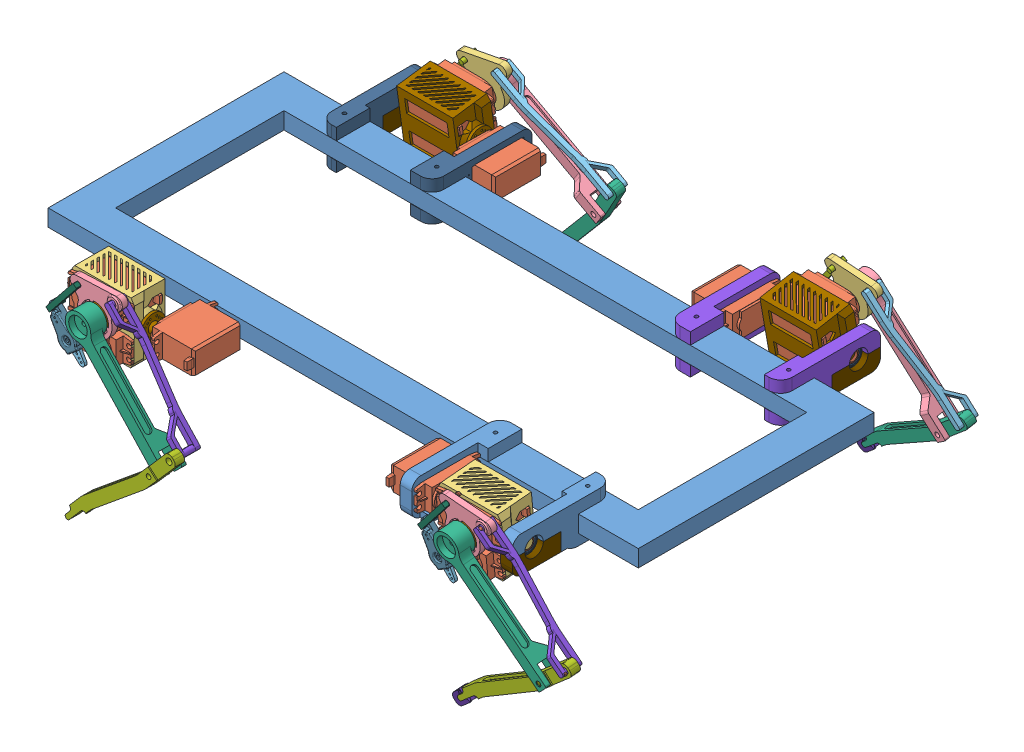
SolidWorks assembly Main Robot Assembly, configuration Default. Lengths in mm.
Overall size (614.33 209.08 462.35).
127 component instances, 28 part files, 12 mates.
Components (placement in the parent):
- Canvas Dimensions-1: Canvas Dimensions [Default] at (344.428 262.5412 316.9027) size (508 14.5 203)
- Robot Assembly-1: Robot Assembly [Default] at (-142.6556 246.9594 574.0725) x (-1 0 0) z (0 0.999972 -0.007524) size (279.4 91.93 183.61) (flexible)
  - MG996R-1: MG996R [Default] at (-78.3336 -28.8336 37.8009) size (54.5 42.75 20)
  - MG996R-2: MG996R [Default] at (-78.3336 -28.8336 11.8009) x (-1 0 0) z (0 0 -1) size (54.5 42.75 20)
  - MG996R-3: MG996R [Default] at (-152.8336 -26.2341 24.7786) x (0 -0.999972 0.007524) z (0 0.007524 0.999972) size (54.5 42.75 20)
  - Servo Housing-1: Servo Housing [Default] at (-78.3336 0.9164 37.8009) x (1 0 0) z (0 1 0) size (61.5 52 29.25)
  - Rotating Piece-1: Rotating Piece [Default] at (-88.8336 10.9164 37.9023) x (0.272127 0 -0.962261) z (0.962261 0 0.272127) size (44.28 6 43.21)
  - Double_Blade_Rudder-1: Double_Blade_Rudder [默认] at (-67.8336 16.2164 11.6996) x (0.777995 0 -0.62827) z (-0.62827 0 -0.777995) size (12.2 5.5 38)
  - Upper Leg-1: Upper Leg [Default] at (-164.7696 20.2164 -34.7892) x (-0.725082 0 0.688662) z (0 1 0) size (22 116.4 18)
  - Lower leg-1: Lower leg [Default] at (-80.9738 38.0729 -100.4378) x (0.753928 0 0.656957) z (0 -1 0) size (20.21 126 9.59)
  - Long Connection Rod-1: Long Connection Rod [Default] at (-101.7266 10.9164 56.8385) x (0.725085 0 -0.688659) z (-0.688659 0 -0.725085) size (5 22 105.4)
  - Circle Rudder-1: Circle Rudder [默认] at (-105.5836 -15.7336 24.8009) x (0 0.704253 -0.709949) z (0 0.709949 0.704253) size (20.8 5.5 20.8)
  - 688ZZ Bearing Assembly-2: 688ZZ Bearing Assembly [Default] at (-46.5836 -15.7336 24.8009) x (0 -0.986239 -0.165327) z (1 0 0) size (17.99 17.98 5)
    - Outer Ring-1: Outer Ring [Default] at origin size (16 16 5)
    - Inner Ring-1: Inner Ring [Default] x (-0.241565 -0.970385 0) z (0 0 1) size (10.6 10.6 5)
    - Cage-1: Cage [Default] x (0.535517 0.844524 0) z (0 0 1) size (13.01 13.06 2.21)
    - 2mm Ball Bearing-1: 2mm Ball Bearing [Default] at (-5.0671 3.2131 0) x (0.050652 0.835774 0.546732) z (0.977207 -0.154478 0.145614) size (2 2 2)
    - 2mm Ball Bearing-2: 2mm Ball Bearing [Default] at (-5.988 -0.3789 0) x (-0.450278 0.705928 0.546732) z (0.881377 0.449412 0.145614) size (2 2 2)
    - 2mm Ball Bearing-3: 2mm Ball Bearing [Default] at (-4.6217 -3.8262 0) x (-0.779216 0.306441 0.546732) z (0.448891 0.881642 0.145614) size (2 2 2)
    - 2mm Ball Bearing-4: 2mm Ball Bearing [Default] at (-1.49 -5.812 0) x (-0.810521 -0.210096 0.546732) z (-0.155056 0.977115 0.145614) size (2 2 2)
    - 2mm Ball Bearing-5: 2mm Ball Bearing [Default] at (2.2108 -5.5778 0) x (-0.532234 -0.646383 0.546732) z (-0.699777 0.699363 0.145614) size (2 2 2)
    - 2mm Ball Bearing-6: 2mm Ball Bearing [Default] at (5.0671 -3.2131 0) x (-0.050652 -0.835774 0.546732) z (-0.977207 0.154478 0.145614) size (2 2 2)
    - 2mm Ball Bearing-7: 2mm Ball Bearing [Default] at (5.988 0.3789 0) x (0.450278 -0.705928 0.546732) z (-0.881377 -0.449412 0.145614) size (2 2 2)
    - 2mm Ball Bearing-8: 2mm Ball Bearing [Default] at (4.6217 3.8262 0) x (0.779216 -0.306441 0.546732) z (-0.448891 -0.881642 0.145614) size (2 2 2)
    - 2mm Ball Bearing-9: 2mm Ball Bearing [Default] at (1.49 5.812 0) x (0.810521 0.210096 0.546732) z (0.155056 -0.977115 0.145614) size (2 2 2)
    - 2mm Ball Bearing-10: 2mm Ball Bearing [Default] at (-2.2108 5.5778 0) x (0.532234 0.646383 0.546732) z (0.699777 -0.699363 0.145614) size (2 2 2)
  - Circle Rudder-3: Circle Rudder [默认] at (-88.8336 16.2164 37.9023) x (-0.701297 0 -0.712869) z (-0.712869 0 0.701297) size (20.8 5.5 20.8)
  - Servo Arm Mount-1: Servo Arm Mount [Default] at (-67.8336 16.2164 11.6996) x (-0.777995 0 0.62827) z (0 1 0) size (16.2 34.39 7.06)
  - Short Connecting Rod-1: Short Connecting Rod [Default] at (-51.1485 16.2164 29.347) x (-0.625385 0 0.780316) z (0 1 0) size (37.08 4 13)
  - 91595A167_Dowel Pin-1: 91595A167_Dowel Pin [91595A167] at (-157.9784 20.8164 -34.8994) x (-0.98004 0 -0.198802) z (0 -1 0) size (4 4 20)
- Rear Robot Assembly-1: Rear Robot Assembly [Default] at (318.8891 198.8409 650.2972) x (-0.962615 -0.122983 0.241344) z (-0.105199 0.990787 0.085287) size (170.41 148.65 173.65) (flexible)
  - MG996R-1: MG996R [Default] at (29.5952 -122.5628 58.2658) x (-0.962615 0.249609 -0.105199) z (0.100626 -0.031047 -0.99444) size (54.5 42.75 20)
  - MG996R-2: MG996R [Default] at (26.9789 -121.7556 84.1213) x (0.962615 -0.249609 0.105199) z (-0.100626 0.031047 0.99444) size (54.5 42.75 20)
  - MG996R-3: MG996R [Default] at (100.7498 -138.2322 78.1733) x (-0.241344 -0.966685 -0.085287) z (0.122983 0.056709 -0.990787) size (54.5 42.75 20)
  - Servo Housing-1: Servo Housing [Default] at (37.077 -93.7693 58.1239) x (-0.962615 0.249609 -0.105199) z (0.251487 0.967849 -0.00477) size (61.5 52 29.25)
  - Rotating Piece-1: Rotating Piece [Default] at (26.8579 -80.6595 82.9278) x (0.47519 -0.127764 -0.870558) z (0.843178 -0.216668 0.492043) size (44.28 6 43.21)
  - Double_Blade_Rudder-1: Double_Blade_Rudder [默认] at (51.0424 -81.5852 59.0548) x (0.874959 -0.229452 -0.426377) z (-0.413763 0.103055 -0.904533) size (12.2 5.5 38)
  - Upper Leg-1: Upper Leg [Default] at (-40.9774 -53.7999 6.6799) x (-0.731758 0.193362 0.65356) z (0.251487 0.967849 -0.00477) size (22 116.4 18)
  - Lower leg-1: Lower leg [Default] at (54.3425 -73.1084 -38.5951) x (0.559538 -0.141367 0.816659) z (-0.251487 -0.967849 0.00477) size (20.21 126 9.59)
  - Long Connection Rod-1: Long Connection Rod [Default] at (10.5252 -76.3432 97.6098) x (0.731755 -0.193361 -0.653564) z (-0.633473 0.160873 -0.756856) size (5 22 105.4)
  - Circle Rudder-1: Circle Rudder [默认] at (57.8128 -116.2822 73.9977) x (0.107242 0.707834 0.698191) z (0.248738 0.660808 -0.70814) size (20.8 5.5 20.8)
  - 688ZZ Bearing Assembly-2: 688ZZ Bearing Assembly [Default] at (1.0185 -101.5553 67.791) x (-0.264501 -0.949925 0.166376) z (-0.962615 0.249609 -0.105199) size (17.99 17.98 5)
    - Outer Ring-1: Outer Ring [Default] at origin size (16 16 5)
    - Inner Ring-1: Inner Ring [Default] x (-0.241565 -0.970385 0) z (0 0 1) size (10.6 10.6 5)
    - Cage-1: Cage [Default] x (0.535517 0.844524 0) z (0 0 1) size (13.01 13.06 2.21)
    - 2mm Ball Bearing-1: 2mm Ball Bearing [Default] at (-5.0671 3.2131 0) x (0.050652 0.835774 0.546732) z (0.977207 -0.154478 0.145614) size (2 2 2)
    - 2mm Ball Bearing-2: 2mm Ball Bearing [Default] at (-5.988 -0.3789 0) x (-0.450278 0.705928 0.546732) z (0.881377 0.449412 0.145614) size (2 2 2)
    - 2mm Ball Bearing-3: 2mm Ball Bearing [Default] at (-4.6217 -3.8262 0) x (-0.779216 0.306441 0.546732) z (0.448891 0.881642 0.145614) size (2 2 2)
    - 2mm Ball Bearing-4: 2mm Ball Bearing [Default] at (-1.49 -5.812 0) x (-0.810521 -0.210096 0.546732) z (-0.155056 0.977115 0.145614) size (2 2 2)
    - 2mm Ball Bearing-5: 2mm Ball Bearing [Default] at (2.2108 -5.5778 0) x (-0.532234 -0.646383 0.546732) z (-0.699777 0.699363 0.145614) size (2 2 2)
    - 2mm Ball Bearing-6: 2mm Ball Bearing [Default] at (5.0671 -3.2131 0) x (-0.050652 -0.835774 0.546732) z (-0.977207 0.154478 0.145614) size (2 2 2)
    - 2mm Ball Bearing-7: 2mm Ball Bearing [Default] at (5.988 0.3789 0) x (0.450278 -0.705928 0.546732) z (-0.881377 -0.449412 0.145614) size (2 2 2)
    - 2mm Ball Bearing-8: 2mm Ball Bearing [Default] at (4.6217 3.8262 0) x (0.779216 -0.306441 0.546732) z (-0.448891 -0.881642 0.145614) size (2 2 2)
    - 2mm Ball Bearing-9: 2mm Ball Bearing [Default] at (1.49 5.812 0) x (0.810521 0.210096 0.546732) z (0.155056 -0.977115 0.145614) size (2 2 2)
    - 2mm Ball Bearing-10: 2mm Ball Bearing [Default] at (-2.2108 5.5778 0) x (0.532234 0.646383 0.546732) z (0.699777 -0.699363 0.145614) size (2 2 2)
  - Circle Rudder-3: Circle Rudder [默认] at (28.1908 -75.5299 82.9026) x (0.821577 -0.21087 0.529666) z (0.511631 -0.137123 -0.848193) size (20.8 5.5 20.8)
  - Servo Arm Mount-1: Servo Arm Mount [Default] at (51.0424 -81.5852 59.0548) x (-0.874959 0.229452 0.426377) z (0.251487 0.967849 -0.00477) size (16.2 34.39 7.06)
  - Short Connecting Rod-1: Short Connecting Rod [Default] at (62.7824 -84.5334 79.8218) x (-0.680527 0.180329 0.710186) z (0.251487 0.967849 -0.00477) size (37.08 4 13)
  - 91595A167_Dowel Pin-1: 91595A167_Dowel Pin [91595A167] at (-34.4066 -55.5062 6.8913) x (-0.945505 0.244623 -0.214897) z (-0.251487 -0.967849 0.00477) size (4 4 20)
  - Foot Cap-1: Foot Cap [Default] at (37.6943 -68.7692 -38.6824) x (0.559538 -0.141367 0.816659) z (-0.251487 -0.967849 0.00477) size (10.5 14 9.53)
  - Lower Leg Mount-1: Lower Leg Mount [Default] at (-1.6759 -81.5579 68.6011) x (0.241344 0.966685 0.085287) z (0.962615 -0.249609 0.105199) size (41.75 15.4 10)
  - Reverse Side Leg Mount-1: Reverse Side Leg Mount [Default] at (-136.4701 -136.4866 64.2689) x (0.241344 0.966685 0.085287) z (0.962615 -0.249609 0.105199) size (86 33.8 96.5)
  - Rod Cap-1: Rod Cap [Default] at (-53.692 -44.5305 22.1631) x (-0.950455 0.247892 0.187575) z (0.182726 -0.042639 0.982239) size (6.08 7 3)
  - Rod Cap-2: Rod Cap [Default] at (9.1664 -68.546 98.6269) x (-0.316982 0.087019 0.944431) z (0.914481 -0.236001 0.328675) size (6.08 7 3)
  - Rod Cap-3: Rod Cap [Default] at (33.9227 -86.2147 103.9332) x (-0.679633 0.180101 0.7111) z (-0.689096 0.175591 -0.703075) size (6.08 7 3)
- Rear Reverse Robot Assembly-1: Rear Reverse Robot Assembly [Default] at (332.8203 121.1113 275.4254) x (0.091818 0.120884 0.988411) z (-0.992282 0.094184 0.080659) size (151.17 176.28 178.68) (flexible)
  - RearRotatingPiece-1: RearRotatingPiece [Default] at (12.4494 157.1176 85.7417) x (-0.304366 -0.905367 0.296095) z (0.031686 0.301047 0.953083) size (44.28 6 43.21)
  - RearUpperLeg-1: RearUpperLeg [Default] at (-6.6252 85.2078 11.4642) x (0.246299 0.627814 -0.738367) z (0.952028 -0.299468 0.062941) size (22 116.4 18)
  - RearLongConnectingRod-1: RearLongConnectingRod [Default] at (-32.961 190.8855 68.9711) x (-0.246298 -0.627811 0.73837) z (-0.181603 -0.718451 -0.671452) size (5 22 107.31)
  - RearLowerLeg-1: RearLowerLeg [Default] at (-26.5278 24.8928 97.0279) x (0.158617 0.658815 0.735394) z (-0.952028 0.299468 -0.062941) size (20.21 126 9.59)
  - RearShortConnectingRod-1: RearShortConnectingRod [Default] at (18.9646 143.6981 120.356) x (0.286718 0.801059 -0.52545) z (0.952028 -0.299468 0.062941) size (37.08 4 13)
  - Circle Rudder-1: Circle Rudder [默认] at (11.4281 139.3867 122.2016) x (0.455641 -0.889568 -0.032554) z (-0.885415 -0.449136 -0.119653) size (20.8 5.5 20.8)
  - Double_Blade_Rudder-1: Double_Blade_Rudder [默认] at (-21.5524 137.6171 102.1209) x (-0.226294 -0.550514 0.80357) z (0.205994 0.779265 0.591873) size (12.2 5.5 38)
  - 688ZZ Bearing Assembly-1: 688ZZ Bearing Assembly [Default] at (17.0351 144.3872 61.4644) x (0.995768 -0.003841 0.091818) z (-0.091818 -0.083342 0.992282) size (17.99 17.98 5)
    - Outer Ring-1: Outer Ring [Default] at origin size (16 16 5)
    - Inner Ring-1: Inner Ring [Default] x (-0.241565 -0.970385 0) z (0 0 1) size (10.6 10.6 5)
    - Cage-1: Cage [Default] x (0.535517 0.844524 0) z (0 0 1) size (13.01 13.06 2.21)
    - 2mm Ball Bearing-1: 2mm Ball Bearing [Default] at (-5.0671 3.2131 0) x (0.050652 0.835774 0.546732) z (0.977207 -0.154478 0.145614) size (2 2 2)
    - 2mm Ball Bearing-2: 2mm Ball Bearing [Default] at (-5.988 -0.3789 0) x (-0.450278 0.705928 0.546732) z (0.881377 0.449412 0.145614) size (2 2 2)
    - 2mm Ball Bearing-3: 2mm Ball Bearing [Default] at (-4.6217 -3.8262 0) x (-0.779216 0.306441 0.546732) z (0.448891 0.881642 0.145614) size (2 2 2)
    - 2mm Ball Bearing-4: 2mm Ball Bearing [Default] at (-1.49 -5.812 0) x (-0.810521 -0.210096 0.546732) z (-0.155056 0.977115 0.145614) size (2 2 2)
    - 2mm Ball Bearing-5: 2mm Ball Bearing [Default] at (2.2108 -5.5778 0) x (-0.532234 -0.646383 0.546732) z (-0.699777 0.699363 0.145614) size (2 2 2)
    - 2mm Ball Bearing-6: 2mm Ball Bearing [Default] at (5.0671 -3.2131 0) x (-0.050652 -0.835774 0.546732) z (-0.977207 0.154478 0.145614) size (2 2 2)
    - 2mm Ball Bearing-7: 2mm Ball Bearing [Default] at (5.988 0.3789 0) x (0.450278 -0.705928 0.546732) z (-0.881377 -0.449412 0.145614) size (2 2 2)
    - 2mm Ball Bearing-8: 2mm Ball Bearing [Default] at (4.6217 3.8262 0) x (0.779216 -0.306441 0.546732) z (-0.448891 -0.881642 0.145614) size (2 2 2)
    - 2mm Ball Bearing-9: 2mm Ball Bearing [Default] at (1.49 5.812 0) x (0.810521 0.210096 0.546732) z (0.155056 -0.977115 0.145614) size (2 2 2)
    - 2mm Ball Bearing-10: 2mm Ball Bearing [Default] at (-2.2108 5.5778 0) x (0.532234 0.646383 0.546732) z (0.699777 -0.699363 0.145614) size (2 2 2)
  - Lower Leg Mount-1: Lower Leg Mount [Default] at (-1.7272 146.59 62.4328) x (-0.988411 0.128599 -0.080659) z (0.091818 0.083342 -0.992282) size (41.75 15.4 10)
  - MG996R-3: MG996R [Default] at (17.6577 134.1817 167.7413) x (0.988411 -0.128599 0.080659) z (0.120884 0.988188 0.094184) size (54.5 42.75 20)
  - Circle Rudder-2: Circle Rudder [默认] at (-11.6369 164.6942 84.1493) x (-0.290319 -0.81888 0.495127) z (0.096734 0.489648 0.866538) size (20.8 5.5 20.8)
  - MG996R-4: MG996R [Default] at (22.4614 124.845 94.5392) x (0.091818 0.083342 -0.992282) z (0.291911 0.950459 0.106841) size (54.5 42.75 20)
  - MG996R-5: MG996R [Default] at (30.3175 150.4244 97.4146) x (-0.091818 -0.083342 0.992282) z (-0.291911 -0.950459 -0.106841) size (54.5 42.75 20)
  - Servo Arm Mount-1: Servo Arm Mount [Default] at (-21.6476 137.647 102.1146) x (-0.226294 -0.550514 0.80357) z (-0.952028 0.299468 -0.062941) size (16.2 34.39 7.06)
  - Foot Cap-1: Foot Cap [Default] at (-52.0591 36.651 78.4027) x (0.158617 0.658815 0.735394) z (-0.952028 0.299468 -0.062941) size (10.5 14 9.53)
  - Rear Reverse eg Mount-1: Rear Reverse eg Mount [Default] at (-93.0222 185.9824 -70.1903) x (0.988411 -0.128599 0.080659) z (-0.091818 -0.083342 0.992282) size (86 33.8 96.5)
  - RearServoHousing-1: RearServoHousing [Default] at (-19.1561 90.4667 87.8008) x (0.091818 0.083342 -0.992282) z (-0.952028 0.299468 -0.062941) size (61.5 52 29.25)
- Reverse Robot Assembly-2: Reverse Robot Assembly [Default] at (30.3159 213.6541 311.9399) x (0 0 1) z (-1 0 0) size (126.32 172.64 154.15) (flexible)
  - RearLegMount-1: RearLegMount [Default] at (-158.0372 73.3871 37.3879) size (86 33.8 96.5)
  - RearRotatingPiece-1: RearRotatingPiece [Default] at (-38.0357 72.1303 81.9379) x (-0.136898 -0.98514 0.10372) z (0.014276 0.102733 0.994606) size (44.28 6 43.21)
  - RearUpperLeg-1: RearUpperLeg [Default] at (-47.0234 16.8987 -7.0604) x (0.112914 0.812552 -0.571847) z (0.990482 -0.13764 0) size (22 116.4 18)
  - RearLongConnectingRod-1: RearLongConnectingRod [Default] at (-89.0615 100.1739 72.4523) x (-0.112914 -0.812551 0.571849) z (-0.078709 -0.566407 -0.820359) size (5 22 107.31)
  - RearLowerLeg-1: RearLowerLeg [Default] at (-53.4679 -62.1712 64.2449) x (0.071365 0.513552 0.855086) z (-0.990482 0.13764 0) size (20.21 126 9.59)
  - RearShortConnectingRod-1: RearShortConnectingRod [Default] at (-27.3329 59.06 122.1513) x (0.108265 0.779093 -0.617489) z (0.990482 -0.13764 0) size (37.08 4 13)
  - RearServoHousing-2: RearServoHousing [Default] at (-41.658 118.7173 92.4379) x (0 0 1) z (-0.990482 0.13764 0) size (61.5 52 29.25)
  - Circle Rudder-1: Circle Rudder [默认] at (-33.2872 57.9871 65.1879) x (-0.854749 -0.519042 0) z (0.519042 -0.854749 0) size (20.8 5.5 20.8)
  - Double_Blade_Rudder-1: Double_Blade_Rudder [默认] at (-66.9694 49.1844 102.9379) x (-0.101883 -0.733169 0.672371) z (0.092545 0.665971 0.740214) size (12.2 5.5 38)
  - 688ZZ Bearing Assembly-1: 688ZZ Bearing Assembly [Default] at (-33.2872 57.9871 126.3879) size (17.99 17.98 5)
    - Outer Ring-1: Outer Ring [Default] at origin size (16 16 5)
    - Inner Ring-1: Inner Ring [Default] x (-0.241565 -0.970385 0) z (0 0 1) size (10.6 10.6 5)
    - Cage-1: Cage [Default] x (0.535517 0.844524 0) z (0 0 1) size (13.01 13.06 2.21)
    - 2mm Ball Bearing-1: 2mm Ball Bearing [Default] at (-5.0671 3.2131 0) x (0.050652 0.835774 0.546732) z (0.977207 -0.154478 0.145614) size (2 2 2)
    - 2mm Ball Bearing-2: 2mm Ball Bearing [Default] at (-5.988 -0.3789 0) x (-0.450278 0.705928 0.546732) z (0.881377 0.449412 0.145614) size (2 2 2)
    - 2mm Ball Bearing-3: 2mm Ball Bearing [Default] at (-4.6217 -3.8262 0) x (-0.779216 0.306441 0.546732) z (0.448891 0.881642 0.145614) size (2 2 2)
    - 2mm Ball Bearing-4: 2mm Ball Bearing [Default] at (-1.49 -5.812 0) x (-0.810521 -0.210096 0.546732) z (-0.155056 0.977115 0.145614) size (2 2 2)
    - 2mm Ball Bearing-5: 2mm Ball Bearing [Default] at (2.2108 -5.5778 0) x (-0.532234 -0.646383 0.546732) z (-0.699777 0.699363 0.145614) size (2 2 2)
    - 2mm Ball Bearing-6: 2mm Ball Bearing [Default] at (5.0671 -3.2131 0) x (-0.050652 -0.835774 0.546732) z (-0.977207 0.154478 0.145614) size (2 2 2)
    - 2mm Ball Bearing-7: 2mm Ball Bearing [Default] at (5.988 0.3789 0) x (0.450278 -0.705928 0.546732) z (-0.881377 -0.449412 0.145614) size (2 2 2)
    - 2mm Ball Bearing-8: 2mm Ball Bearing [Default] at (4.6217 3.8262 0) x (0.779216 -0.306441 0.546732) z (-0.448891 -0.881642 0.145614) size (2 2 2)
    - 2mm Ball Bearing-9: 2mm Ball Bearing [Default] at (1.49 5.812 0) x (0.810521 0.210096 0.546732) z (0.155056 -0.977115 0.145614) size (2 2 2)
    - 2mm Ball Bearing-10: 2mm Ball Bearing [Default] at (-2.2108 5.5778 0) x (0.532234 0.646383 0.546732) z (0.699777 -0.699363 0.145614) size (2 2 2)
  - Lower Leg Mount-1: Lower Leg Mount [Default] at (-52.0372 57.9871 133.8879) x (-1 0 0) z (0 0 -1) size (41.75 15.4 10)
  - MG996R-3: MG996R [Default] at (-22.7872 58.4435 20.1379) x (1 0 0) z (0 -1 0) size (54.5 42.75 20)
  - Circle Rudder-2: Circle Rudder [默认] at (-63.0949 75.6126 81.9379) x (-0.120143 -0.864571 0.487937) z (0.06716 0.483293 0.872879) size (20.8 5.5 20.8)
  - MG996R-4: MG996R [Default] at (-22.164 42.8558 92.4379) x (0 0 -1) z (0.13764 0.990482 0) size (54.5 42.75 20)
  - MG996R-5: MG996R [Default] at (-18.4598 69.5123 92.4379) x (0 0 1) z (-0.13764 -0.990482 0) size (54.5 42.75 20)
  - Servo Arm Mount-1: Servo Arm Mount [Default] at (-67.0685 49.1981 102.9379) x (-0.101883 -0.733169 0.672371) z (-0.990482 0.13764 0) size (16.2 34.39 7.06)
  - Foot Cap-1: Foot Cap [Default] at (-81.2578 -51.4579 48.4352) x (0.071365 0.513552 0.855086) z (-0.990482 0.13764 0) size (10.5 14 9.53)
Mates (geometry in assembly coordinates):
- Coincident1: coincident anti-aligned: plane of Canvas Dimensions-1 through (344.428 277.0412 519.9027) normal (0 0 1); plane of Robot Assembly-1/Leg Mount-1 through (-103.572 262.2412 519.9027) normal (0 0 -1)
- Coincident2: coincident anti-aligned: plane of Canvas Dimensions-1 through (344.428 277.0412 316.9027) normal (0 1 0); plane of Robot Assembly-1/Leg Mount-1 through (-103.572 277.0412 519.9027) normal (0 -1 0)
- Distance1: distance = 60 mm: plane of Robot Assembly-1/Leg Mount-1 through (-103.572 287.0412 490.9027) normal (-1 0 0); plane of Canvas Dimensions-1 through (-163.572 277.0412 316.9027) normal (-1 0 0)
- Coincident15: coincident anti-aligned: plane of Canvas Dimensions-1 through (344.428 277.0412 316.9027) normal (0 1 0); plane of Rear Robot Assembly-1/Reverse Side Leg Mount-1 through (292.928 277.0412 519.9027) normal (0 -1 0)
- Coincident16: coincident anti-aligned: plane of Canvas Dimensions-1 through (344.428 277.0412 519.9027) normal (0 0 1); plane of Rear Robot Assembly-1/Reverse Side Leg Mount-1 through (292.928 262.2412 519.9027) normal (0 0 -1)
- Distance4: distance = 300 mm: plane of Rear Robot Assembly-1/Reverse Side Leg Mount-1 through (196.428 287.0412 490.9027) normal (-1 0 0); plane of Robot Assembly-1/Leg Mount-1 through (-103.572 287.0412 490.9027) normal (-1 0 0)
- Coincident18: coincident anti-aligned: plane of Canvas Dimensions-1 through (344.428 277.0412 316.9027) normal (0 0 -1); plane of Rear Reverse Robot Assembly-1/Rear Reverse eg Mount-1 through (292.928 262.2412 316.9027) normal (0 0 1)
- Coincident19: coincident anti-aligned: plane of Canvas Dimensions-1 through (344.428 277.0412 316.9027) normal (0 1 0); plane of Rear Reverse Robot Assembly-1/Rear Reverse eg Mount-1 through (292.928 277.0412 316.9027) normal (0 -1 0)
- Coincident20: coincident aligned: plane of Rear Robot Assembly-1/Reverse Side Leg Mount-1 through (196.428 287.0412 490.9027) normal (-1 0 0); plane of Rear Reverse Robot Assembly-1/Rear Reverse eg Mount-1 through (196.428 287.0412 345.9027) normal (-1 0 0)
- Coincident21: coincident anti-aligned: plane of Canvas Dimensions-1 through (344.428 277.0412 316.9027) normal (0 0 -1); plane of Reverse Robot Assembly-2/RearLegMount-1 through (-103.572 262.2412 316.9027) normal (0 0 1)
- Coincident22: coincident anti-aligned: plane of Canvas Dimensions-1 through (344.428 277.0412 316.9027) normal (0 1 0); plane of Reverse Robot Assembly-2/RearLegMount-1 through (-103.572 277.0412 316.9027) normal (0 -1 0)
- Coincident23: coincident: plane of Robot Assembly-1/Leg Mount-1 through (-7.072 287.0412 490.9027) normal (1 0 0); plane of Reverse Robot Assembly-2/RearLegMount-1 through (-7.072 287.0412 345.9027) normal (1 0 0)
